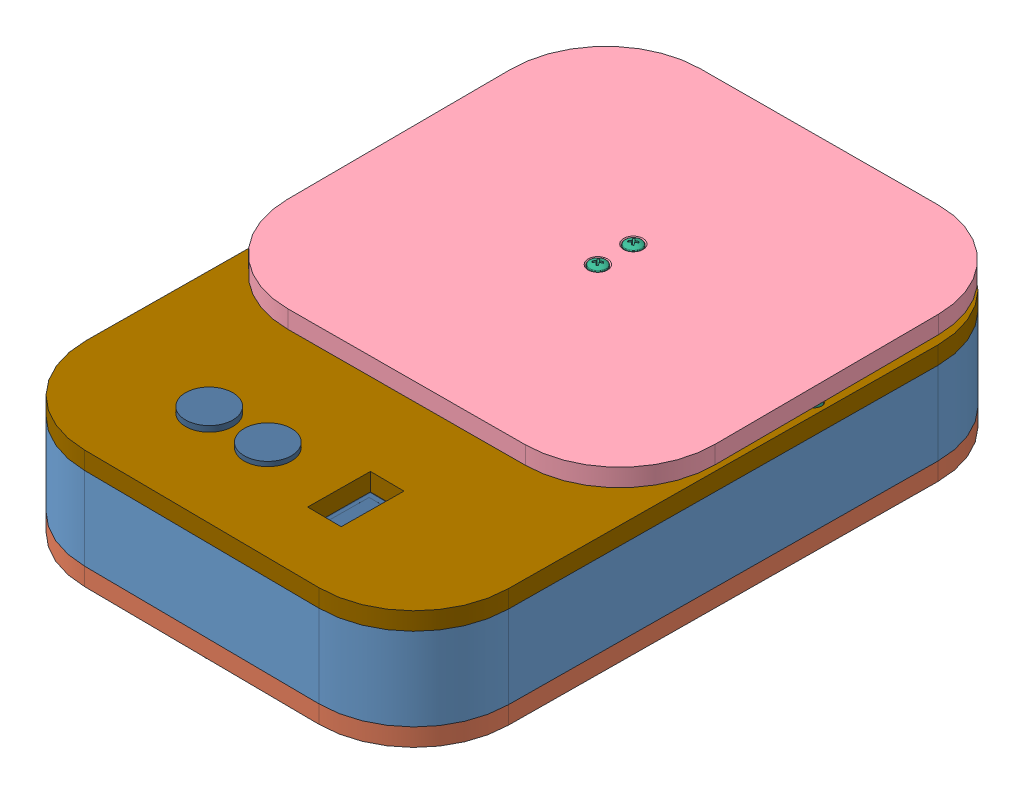
SolidWorks assembly Mainv2.0, configuration Default. Lengths in mm.
Overall size (189.49 80.65 261.56).
193 component instances, 46 part files, 22 mates.
Components (placement in the parent):
- Main-1: Main [Default] at (-331.7007 96.9527 454.1899) size (182.26 61.96 261.56)
  - mail wall-1: mail wall [Default] at (468.1099 74.0645 -181.95) x (-0.999962 0 -0.008727) z (0.008727 0 -0.999962) size (180 35 260)
  - bottom lid-2: bottom lid [Default] at (468.1099 31.5645 -181.95) x (0.999962 0 0.008727) z (-0.008727 0 0.999962) size (180 7.5 260)
  - Loadcell-1kg-No Name.step-1: Loadcell-1kg-No Name.step [Default] at (468.4825 94.8439 -197.5959) x (0 0 1) z (-1 0 0) size (91.8 14.23 13.91)
  - tray-1: tray [Default] at (468.6751 134.9439 -266.3463) x (0.999991 0 -0.00428) z (0.00428 0 0.999991) size (180 7.5 175)
  - Part5-1: Part5 [Default] at origin size (12.6 12.5 27.5)
  - pan cross head_am-1: pan cross head_am [B18.6.7M - M3.5 x 0.6 x 35 Type I Cross Recessed PHMS --35N] at (468.4825 128.4614 -232.8459) x (0 -1 0) z (-0.788636 0 0.61486) size (37.57 7 7)
  - pan cross head_am-3: pan cross head_am [B18.6.7M - M3.5 x 0.6 x 35 Type I Cross Recessed PHMS --35N] at (468.4825 128.5554 -217.8459) x (0 -1 0) z (0.792721 0 -0.609585) size (37.57 7 7)
  - Part1-1: Part1 [Default] at origin size (50 22.7 32.99)
  - hex bolt_am-1: hex bolt_am [B18.2.3.5M - Hex bolt M5 x 0.8 x 35 --16N] at (468.8184 72.2139 -162.6607) x (0 1 0) z (0 0 1) size (38.58 9.24 8)
  - hex bolt_am-2: hex bolt_am [B18.2.3.5M - Hex bolt M5 x 0.8 x 35 --16N] at (468.8184 72.2139 -177.7301) x (0 1 0) z (0 0 1) size (38.58 9.24 8)
  - Top lid with second pcb-2: Top lid with second pcb [Default] at (567.0429 -14.7467 22.0801) x (-0.999962 0 -0.008727) z (0.008727 0 -0.999962) size (180 18.64 260)
    - top lid-1: top lid [Default] at (100.7096 131.3112 203.159) size (180 7.5 260)
    - second_pcb.step-1: second_pcb.step [Default] at (17.5816 118.1729 -168.5329) x (0 0 -1) z (0 1 0) size (33.15 95 11)
    - Part64-1: Part64 [Default] at origin size (95.93 5.6 34.46)
    - pan cross head_am-2: pan cross head_am [B18.6.7M - M4 x 0.7 x 10 Type I Cross Recessed PHMS --10C] at (61.2696 114.6615 128.1391) x (0 1 0) z (0.253418 0 0.967357) size (13.07 8 8)
    - pan cross head_am-3: pan cross head_am [B18.6.7M - M4 x 0.7 x 10 Type I Cross Recessed PHMS --10C] at (152.2016 114.6615 127.7581) x (0 1 0) z (-0.971066 0 -0.238809) size (13.07 8 8)
    - pan cross head_am-4: pan cross head_am [B18.6.7M - M4 x 0.7 x 10 Type I Cross Recessed PHMS --10C] at (152.2016 114.6615 98.6751) x (0 1 0) z (-0.342128 0 -0.939653) size (13.07 8 8)
    - pan cross head_am-5: pan cross head_am [B18.6.7M - M4 x 0.7 x 10 Type I Cross Recessed PHMS --10C] at (61.2696 114.6615 98.6751) x (0 1 0) z (-0.923859 0 -0.382733) size (13.07 8 8)
- pcb_with_screws-1: pcb_with_screws [Default] at (347.1614 488.5879 -158.0964) x (0.371474 0 -0.928443) z (-0.928443 0 -0.371474) size (78.01 61.67 95.13)
  - pcb.step-1: pcb.step [Default] at (-541.6964 307.1593 96.7738) x (-0.93165 0 -0.363358) z (0 -1 0) size (48.01 79.98 16.61)
    - Board.step-1: Board.step [Default] at origin size (48.01 78.74 0.41)
      - Open CASCADE STEP translator 7.5 2.1.1.step-1: Open CASCADE STEP translator 7.5 2.1.1.step [Default] at (0 0 -0.4115) size (48.01 78.74 0.41)
    - HX711 out.step-1: HX711 out.step [Default] at origin size (10.16 2.54 10.59)
      - Header_4.step-1: Header_4.step [Default] at (27.685 46.598 -0.0051) x (0 -1 0) z (-1 0 0) size (2.54 10.59 10.16)
        - header.step-1: header.step [Default] at origin size (2.54 10.59 2.54)
          - header-0.step-1: header-0.step [Default] at origin size (2.54 8.5 2.54)
          - pin.step-1: pin.step [Default] at (-1.4 0 0) size (0.4 10 1.99)
        - header.step-2: header.step [Default] at (0 0 -2.54) size (2.54 10.59 2.54)
          - header-0.step-1: header-0.step [Default] at origin size (2.54 8.5 2.54)
          - pin.step-1: pin.step [Default] at (-1.4 0 0) size (0.4 10 1.99)
        - header.step-3: header.step [Default] at (0 0 -5.08) size (2.54 10.59 2.54)
          - header-0.step-1: header-0.step [Default] at origin size (2.54 8.5 2.54)
          - pin.step-1: pin.step [Default] at (-1.4 0 0) size (0.4 10 1.99)
        - header.step-4: header.step [Default] at (0 0 -7.62) size (2.54 10.59 2.54)
          - header-0.step-1: header-0.step [Default] at origin size (2.54 8.5 2.54)
          - pin.step-1: pin.step [Default] at (-1.4 0 0) size (0.4 10 1.99)
    - HX711_lc.step-1: HX711_lc.step [Default] at origin size (10.16 2.54 10.59)
      - Header_4.step-1: Header_4.step [Default] at (30.23 66.915 -0.0051) x (0 -1 0) z (-1 0 0) size (2.54 10.59 10.16)
        - header.step-1: header.step [Default] at origin size (2.54 10.59 2.54)
          - header-0.step-1: header-0.step [Default] at origin size (2.54 8.5 2.54)
          - pin.step-1: pin.step [Default] at (-1.4 0 0) size (0.4 10 1.99)
        - header.step-2: header.step [Default] at (0 0 -2.54) size (2.54 10.59 2.54)
          - header-0.step-1: header-0.step [Default] at origin size (2.54 8.5 2.54)
          - pin.step-1: pin.step [Default] at (-1.4 0 0) size (0.4 10 1.99)
        - header.step-3: header.step [Default] at (0 0 -5.08) size (2.54 10.59 2.54)
          - header-0.step-1: header-0.step [Default] at origin size (2.54 8.5 2.54)
          - pin.step-1: pin.step [Default] at (-1.4 0 0) size (0.4 10 1.99)
        - header.step-4: header.step [Default] at (0 0 -7.62) size (2.54 10.59 2.54)
          - header-0.step-1: header-0.step [Default] at origin size (2.54 8.5 2.54)
          - pin.step-1: pin.step [Default] at (-1.4 0 0) size (0.4 10 1.99)
    - usb 2.0.step-1: usb 2.0.step [Default] at origin size (7.8 5.5 3.71)
      - USB3090-30-A--3DModel-STEP-56544.step-1: USB3090-30-A--3DModel-STEP-56544.step [Default] at (7.762 1.514 0) x (1 0 0) z (0 -1 0) size (7.8 3.71 5.5)
    - R 470.step-1: R 470.step [Default] at origin size (2 1.25 0.6)
      - 6201218720.step-1: 6201218720.step [Default] at (15.687 7.62 0) x (1 0 0) z (0 0 1) size (2 1.25 0.6)
        - term1.step-1: term1.step [Default] at (-1 -0.625 0) size (0.35 1.25 0.6)
        - term2.step-1: term2.step [Default] at (0.65 -0.625 0) size (0.35 1.25 0.6)
        - body.step-1: body.step [Default] at (-0.65 -0.6125 0.006) size (1.3 1.22 0.59)
    - R 47k.step-1: R 47k.step [Default] at origin size (2 1.25 0.6)
      - 6062674512.step-1: 6062674512.step [Default] at (18.862 49.53 0) x (-1 0 0) z (0 0 1) size (2 1.25 0.6)
        - term1-1.step-1: term1-1.step [Default] at (-1 -0.625 0) size (0.35 1.25 0.6)
        - term2-2.step-1: term2-2.step [Default] at (0.65 -0.625 0) size (0.35 1.25 0.6)
        - body-3.step-1: body-3.step [Default] at (-0.65 -0.6125 0.006) size (1.3 1.22 0.59)
    - R 15k.step-1: R 15k.step [Default] at origin size (2 1.25 0.6)
      - 7267289360.step-1: 7267289360.step [Default] at (18.937 59.563 0) x (-1 0 0) z (0 0 1) size (2 1.25 0.6)
        - solidBody.step-1: solidBody.step [Default] at origin size (1.95 1.25 0.55)
        - Terminal.step-1: Terminal.step [Default] at origin size (2 1.25 0.6)
        - solidTop.step-1: solidTop.step [Default] at origin size (1.2 1.25 0.02)
    - R5-10K.step-1: R5-10K.step [Default] at origin size (1.6 0.8 0.55)
      - CRG0603F10K_10.step-1: CRG0603F10K_10.step [Default] at (45.212 17.526 0) x (1 0 0) z (0 -1 0) size (1.6 0.55 0.8)
    - R4-10K.step-1: R4-10K.step [Default] at origin size (1.6 0.8 0.55)
      - CRG0603F10K_10.step-1: CRG0603F10K_10.step [Default] at (45.212 22.7965 0) x (-1 0 0) z (0 1 0) size (1.6 0.55 0.8)
    - R3-10K.step-1: R3-10K.step [Default] at origin size (1.6 0.8 0.55)
      - CRG0603F10K_10.step-1: CRG0603F10K_10.step [Default] at (45.212 28.067 0) x (1 0 0) z (0 -1 0) size (1.6 0.55 0.8)
    - R 2k.step-1: R 2k.step [Default] at origin size (2 1.25 0.6)
      - 6062674512.step-1: 6062674512.step [Default] at (15.814 12.319 0) x (-1 0 0) z (0 0 1) size (2 1.25 0.6)
        - term1-1.step-1: term1-1.step [Default] at (-1 -0.625 0) size (0.35 1.25 0.6)
        - term2-2.step-1: term2-2.step [Default] at (0.65 -0.625 0) size (0.35 1.25 0.6)
        - body-3.step-1: body-3.step [Default] at (-0.65 -0.6125 0.006) size (1.3 1.22 0.59)
    - R2-10K.step-1: R2-10K.step [Default] at origin size (1.6 0.8 0.55)
      - CRG0603F10K_10.step-1: CRG0603F10K_10.step [Default] at (22.733 36.195 0) x (-1 0 0) z (0 1 0) size (1.6 0.55 0.8)
    - R1-10K.step-1: R1-10K.step [Default] at origin size (1.6 0.8 0.55)
      - CRG0603F10K_10.step-1: CRG0603F10K_10.step [Default] at (22.733 42.545 0) x (-1 0 0) z (0 1 0) size (1.6 0.55 0.8)
    - MCP73831.step-1: MCP73831.step [Default] at origin size (2.7 2.9 1.45)
      - MCP73831T-5ACI_OT.step-1: MCP73831T-5ACI_OT.step [Default] at (8.255 12.012 0) x (0 -1 0) z (-1 0 0) size (2.9 1.45 2.7)
    - LED.step-1: LED.step [Default] at origin size (3 1 2)
      - KPA-3010CGCK-Base.step-1: KPA-3010CGCK-Base.step [Default] at (16.51 1.651 0.508) x (-1 0 0) z (0 0 -1) size (2.16 1 1.02)
      - KPA-3010CGCK-Base-4.step-1: KPA-3010CGCK-Base-4.step [Default] at (16.51 1.651 0.508) x (-1 0 0) z (0 0 -1) size (3 1 1.22)
      - KPA-3010CGCK-Base-5.step-1: KPA-3010CGCK-Base-5.step [Default] at (16.51 1.651 0.508) x (-1 0 0) z (0 0 -1) size (0.9 1 0)
      - KPA-3010CGCK-Base-6.step-1: KPA-3010CGCK-Base-6.step [Default] at (16.51 1.651 0.508) x (-1 0 0) z (0 0 -1) size (0.8 1 0.02)
      - KPA-3010CGCK-Base-7.step-1: KPA-3010CGCK-Base-7.step [Default] at (16.51 1.651 0.508) x (-1 0 0) z (0 0 -1) size (2.96 1 0.96)
    - battery.step-1: battery.step [Default] at origin size (7.4 5.75 10.4)
      - 6062675712.step-1: 6062675712.step [Default] at (9.274 74.295 0) x (1 0 0) z (0 -1 0) size (7.4 10.4 5.75)
    - load cell.step-1: load cell.step [Default] at origin size (10.16 2.54 10.59)
      - Header_4.step-1: Header_4.step [Default] at (30.099 71.755 -0.0051) x (0 -1 0) z (-1 0 0) size (2.54 10.59 10.16)
        - header.step-1: header.step [Default] at origin size (2.54 10.59 2.54)
          - header-0.step-1: header-0.step [Default] at origin size (2.54 8.5 2.54)
          - pin.step-1: pin.step [Default] at (-1.4 0 0) size (0.4 10 1.99)
        - header.step-2: header.step [Default] at (0 0 -2.54) size (2.54 10.59 2.54)
          - header-0.step-1: header-0.step [Default] at origin size (2.54 8.5 2.54)
          - pin.step-1: pin.step [Default] at (-1.4 0 0) size (0.4 10 1.99)
        - header.step-3: header.step [Default] at (0 0 -5.08) size (2.54 10.59 2.54)
          - header-0.step-1: header-0.step [Default] at origin size (2.54 8.5 2.54)
          - pin.step-1: pin.step [Default] at (-1.4 0 0) size (0.4 10 1.99)
        - header.step-4: header.step [Default] at (0 0 -7.62) size (2.54 10.59 2.54)
          - header-0.step-1: header-0.step [Default] at origin size (2.54 8.5 2.54)
          - pin.step-1: pin.step [Default] at (-1.4 0 0) size (0.4 10 1.99)
    - buttons.step-1: buttons.step [Default] at origin size (2.54 10.16 10.59)
      - Header_4.step-1: Header_4.step [Default] at (39.497 59.817 -0.0051) x (-1 0 0) z (0 1 0) size (2.54 10.59 10.16)
        - header.step-1: header.step [Default] at origin size (2.54 10.59 2.54)
          - header-0.step-1: header-0.step [Default] at origin size (2.54 8.5 2.54)
          - pin.step-1: pin.step [Default] at (-1.4 0 0) size (0.4 10 1.99)
        - header.step-2: header.step [Default] at (0 0 -2.54) size (2.54 10.59 2.54)
          - header-0.step-1: header-0.step [Default] at origin size (2.54 8.5 2.54)
          - pin.step-1: pin.step [Default] at (-1.4 0 0) size (0.4 10 1.99)
        - header.step-3: header.step [Default] at (0 0 -5.08) size (2.54 10.59 2.54)
          - header-0.step-1: header-0.step [Default] at origin size (2.54 8.5 2.54)
          - pin.step-1: pin.step [Default] at (-1.4 0 0) size (0.4 10 1.99)
        - header.step-4: header.step [Default] at (0 0 -7.62) size (2.54 10.59 2.54)
          - header-0.step-1: header-0.step [Default] at origin size (2.54 8.5 2.54)
          - pin.step-1: pin.step [Default] at (-1.4 0 0) size (0.4 10 1.99)
    - OLED.step-1: OLED.step [Default] at origin size (2.54 10.16 16)
      - MTSW-104-22-S-S-420.step-1: MTSW-104-22-S-S-420.step [Default] at (44.831 57.277 0) x (0 -1 0) z (-1 0 0) size (10.16 16 2.54)
        - MTSW-104-22-S-420.step-1: MTSW-104-22-S-420.step [Default] at (0 -2.794 0) size (8.51 16 0.89)
        - MTSW-104-22-S-S-420_body.step-1: MTSW-104-22-S-S-420_body.step [Default] at origin size (10.16 2.54 2.54)
    - ESP-12F.step-1: ESP-12F.step [Default] at origin size (17.7 24.9 3.1)
      - ESP-12F-8.step-1: ESP-12F-8.step [Default] at (33.909 28.956 0) x (1 0 0) z (0 -1 0) size (17.7 3.1 24.9)
    - C5-4.7uF.step-1: C5-4.7uF.step [Default] at origin size (2 1.25 1.45)
      - 885012107013.step-1: 885012107013.step [Default] at (10.345 18.923 0) x (-1 0 0) z (0 0 1) size (2 1.25 1.45)
        - Fillet1.step-1: Fillet1.step [Default] at origin size (0.5 1.25 1.45)
        - Fillet2.step-1: Fillet2.step [Default] at origin size (0.5 1.25 1.45)
        - body2.step-1: body2.step [Default] at origin size (1 1.22 1.42)
    - C4-4.7uF.step-1: C4-4.7uF.step [Default] at origin size (2 1.25 1.45)
      - 885012107013.step-1: 885012107013.step [Default] at (11.245 26.543 0) x (1 0 0) z (0 0 1) size (2 1.25 1.45)
        - Fillet1.step-1: Fillet1.step [Default] at origin size (0.5 1.25 1.45)
        - Fillet2.step-1: Fillet2.step [Default] at origin size (0.5 1.25 1.45)
        - body2.step-1: body2.step [Default] at origin size (1 1.22 1.42)
    - C3-10uF.step-1: C3-10uF.step [Default] at origin size (5.3 4.5 5.5)
      - 865080340001.step-1: 865080340001.step [Default] at (10.737 64.643 0) x (-1 0 0) z (0 0 1) size (5.3 4.5 5.5)
        - Base.step-1: Base.step [Default] at origin size (4.5 4.5 1.6)
        - Pin1Fillet.step-1: Pin1Fillet.step [Default] at origin size (2.25 0.75 0.3)
        - Pin2Fillet.step-1: Pin2Fillet.step [Default] at origin size (2.25 0.75 0.3)
        - Fillet.step-1: Fillet.step [Default] at origin size (4.2 4.2 4.4)
      - 865080340001.step-2: 865080340001.step [Default] at (10.737 64.643 0) x (-1 0 0) z (0 0 1) size (5.3 4.5 5.5)
        - Base.step-1: Base.step [Default] at origin size (4.5 4.5 1.6)
        - Pin1Fillet.step-1: Pin1Fillet.step [Default] at origin size (2.25 0.75 0.3)
        - Pin2Fillet.step-1: Pin2Fillet.step [Default] at origin size (2.25 0.75 0.3)
        - Fillet.step-1: Fillet.step [Default] at origin size (4.2 4.2 4.4)
    - C2-10uF.step-1: C2-10uF.step [Default] at origin size (5.3 4.5 5.5)
      - 865080340001.step-1: 865080340001.step [Default] at (10.737 44.069 0) x (-1 0 0) z (0 0 1) size (5.3 4.5 5.5)
        - Base.step-1: Base.step [Default] at origin size (4.5 4.5 1.6)
        - Pin1Fillet.step-1: Pin1Fillet.step [Default] at origin size (2.25 0.75 0.3)
        - Pin2Fillet.step-1: Pin2Fillet.step [Default] at origin size (2.25 0.75 0.3)
        - Fillet.step-1: Fillet.step [Default] at origin size (4.2 4.2 4.4)
      - 865080340001.step-2: 865080340001.step [Default] at (10.737 44.069 0) x (-1 0 0) z (0 0 1) size (5.3 4.5 5.5)
        - Base.step-1: Base.step [Default] at origin size (4.5 4.5 1.6)
        - Pin1Fillet.step-1: Pin1Fillet.step [Default] at origin size (2.25 0.75 0.3)
        - Pin2Fillet.step-1: Pin2Fillet.step [Default] at origin size (2.25 0.75 0.3)
        - Fillet.step-1: Fillet.step [Default] at origin size (4.2 4.2 4.4)
    - C1-10uF.step-1: C1-10uF.step [Default] at origin size (5.3 4.5 5.5)
      - 865080340001.step-1: 865080340001.step [Default] at (33.583 11.303 0) x (-1 0 0) z (0 0 1) size (5.3 4.5 5.5)
        - Base.step-1: Base.step [Default] at origin size (4.5 4.5 1.6)
        - Pin1Fillet.step-1: Pin1Fillet.step [Default] at origin size (2.25 0.75 0.3)
        - Pin2Fillet.step-1: Pin2Fillet.step [Default] at origin size (2.25 0.75 0.3)
        - Fillet.step-1: Fillet.step [Default] at origin size (4.2 4.2 4.4)
      - 865080340001.step-2: 865080340001.step [Default] at (33.583 11.303 0) x (-1 0 0) z (0 0 1) size (5.3 4.5 5.5)
        - Base.step-1: Base.step [Default] at origin size (4.5 4.5 1.6)
        - Pin1Fillet.step-1: Pin1Fillet.step [Default] at origin size (2.25 0.75 0.3)
        - Pin2Fillet.step-1: Pin2Fillet.step [Default] at origin size (2.25 0.75 0.3)
        - Fillet.step-1: Fillet.step [Default] at origin size (4.2 4.2 4.4)
    - TC2117.step-1: TC2117.step [Default] at origin size (7.13 5.32 1.17)
      - TC2117-3.3VDBTR.step-1: TC2117-3.3VDBTR.step [Default] at (10.864 54.356 0) x (-1 0 0) z (0 0 1) size (7 5.32 1.17)
        - body.step-1: body.step [Default] at origin size (1.3 1.22 0.59)
        - PinsArrayL.step-1: PinsArrayL.step [Default] at origin size (1.75 5.32 1.17)
        - FilletPinR.step-1: FilletPinR.step [Default] at origin size (1.75 3 1.17)
      - TC2117-3.3VDBTR.step-2: TC2117-3.3VDBTR.step [Default] at (10.737 54.356 0) x (-1 0 0) z (0 0 1) size (7 5.32 1.17)
        - body.step-1: body.step [Default] at origin size (1.3 1.22 0.59)
        - PinsArrayL.step-1: PinsArrayL.step [Default] at origin size (1.75 5.32 1.17)
        - FilletPinR.step-1: FilletPinR.step [Default] at origin size (1.75 3 1.17)
  - Part36-1: Part36 [Default] at (-868.0076 716.489 235.6311) x (0.932186 0.214397 0.291656) z (-0.265595 0.952553 0.148668) size (53.08 79 35.65)
  - pan cross head_am-4: pan cross head_am [B18.6.7M - M2.5 x 0.45 x 5 Type I Cross Recessed PHMS --5N] at (-581.9119 305.0593 74.4096) x (0 1 0) z (-0.92188 0 0.387475) size (7.07 5 5)
  - pan cross head_am-5: pan cross head_am [B18.6.7M - M2.5 x 0.45 x 5 Type I Cross Recessed PHMS --5N] at (-556.4391 305.0593 9.0972) x (0 1 0) z (-0.72878 0 -0.684748) size (7.07 5 5)
  - pan cross head_am-6: pan cross head_am [B18.6.7M - M2.5 x 0.45 x 5 Type I Cross Recessed PHMS --5N] at (-515.9277 305.0593 24.761) x (0 1 0) z (0.615507 0 -0.788131) size (7.07 5 5)
  - pan cross head_am-7: pan cross head_am [B18.6.7M - M2.5 x 0.45 x 5 Type I Cross Recessed PHMS --5N] at (-541.4467 305.0593 90.1917) x (0 1 0) z (-0.986634 0 -0.162951) size (7.07 5 5)
- Part37^Mainv2.0-1: Part37^Mainv2.0 [Default] at (232.9335 200.1845 720.6732) x (-0.999475 0 0.032385) z (0 1 0) size (19.97 19.97 10) (virtual)
- Part37^Mainv2.0-2: Part37^Mainv2.0 [Default] at (177.4351 200.668 728.4104) x (-0.998664 0 -0.051668) z (0 1 0) size (19.97 19.97 10) (virtual)
- pan cross head_am-3: pan cross head_am [B18.6.7M - M3 x 0.5 x 16 Type I Cross Recessed PHMS --16C] at (137.5058 161.1172 146.5823) x (0 1 0) z (0 0 1) size (18.37 5.6 5.6)
- pan cross head_am-4: pan cross head_am [B18.6.7M - M3 x 0.5 x 16 Type I Cross Recessed PHMS --16C] at (50.1199 161.1172 271.4869) x (0 1 0) z (0 0 1) size (18.37 5.6 5.6)
- pan cross head_am-7: pan cross head_am [B18.6.7M - M3 x 0.5 x 16 Type I Cross Recessed PHMS --16C] at (222.0917 161.1172 272.9876) x (0 1 0) z (0 0 1) size (18.37 5.6 5.6)
- pan cross head_am-9: pan cross head_am [B18.6.7M - M3 x 0.5 x 16 Type I Cross Recessed PHMS --16C] at (135.3113 161.1172 398.0567) x (0 1 0) z (0 0 1) size (18.37 5.6 5.6)
- pan cross head_am-11: pan cross head_am [B18.6.7M - M3 x 0.5 x 16 Type I Cross Recessed PHMS --16C] at (52.0363 215.7083 230.7075) x (0 -1 0) z (0.190223 0 -0.981741) size (18.37 5.6 5.6)
- pan cross head_am-13: pan cross head_am [B18.6.7M - M3 x 0.5 x 16 Type I Cross Recessed PHMS --16C] at (221.8864 215.4097 229.9805) x (0 -1 0) z (-0.613644 0 -0.789583) size (18.37 5.6 5.6)
- pan cross head_am-14: pan cross head_am [B18.6.7M - M3 x 0.5 x 16 Type I Cross Recessed PHMS --16C] at (137.5433 215.6271 147.9494) x (0 -1 0) z (0.848821 0 -0.52868) size (18.37 5.6 5.6)
Mates (geometry in assembly coordinates):
- Coincident1: coincident anti-aligned: plane of Main-1/bottom lid-2 through (85.6258 171.0172 361.8002) normal (0 1 0); circle of pcb_with_screws-1/Part36-1
- Coincident2: coincident anti-aligned: plane of Main-1/mail wall-1 through (55.3651 206.0172 391.5372) normal (0.999962 0 0.008727); plane of pcb_with_screws-1/pcb.step-1/Board.step-1/Open CASCADE STEP translator 7.5 2.1.1.step-1 through (56.0864 181.0172 308.8891) normal (-0.999962 0 -0.008727)
- Lock1: lock: unknown of Main-1/bottom lid-2; unknown of pcb_with_screws-1/Part36-1
- Concentric4: concentric anti-aligned: circle of Main-1/top lid-1; circle of Part37^Mainv1.1-2
- Concentric5: concentric anti-aligned: circle of Main-1/top lid-1; circle of Part37^Mainv1.1-1
- Concentric7: concentric aligned: cylinder of Main-1/bottom lid-2 through (222.0917 163.5172 272.9876) axis (0 -1 0) radius 1.7; cylinder of pan cross head_am-4 through (222.0917 109.9845 272.9876) axis (0 -1 0) radius 1.5
- Concentric8: concentric anti-aligned: circle of Main-1/Top lid with second pcb-2/top lid-1; circle of Part37^Mainv2.0-1
- Concentric9: concentric anti-aligned: circle of Main-1/Top lid with second pcb-2/top lid-1; circle of Part37^Mainv2.0-2
- Concentric10: concentric anti-aligned: cone of Main-1/bottom lid-2 through (137.5058 163.5172 146.5823) axis (0 1 0); cylinder of pan cross head_am-3 through (137.5058 135.7172 146.5823) axis (0 -1 0) radius 2.8
- Coincident4: coincident anti-aligned: plane of Main-1/bottom lid-2 through (85.6258 163.5172 361.8002) normal (0 -1 0); plane of pan cross head_am-3 through (136.0058 163.5172 146.5823) normal (0 1 0)
- Concentric11: concentric anti-aligned: cone of Main-1/bottom lid-2 through (50.1199 163.5172 271.4869) axis (0 1 0); cylinder of pan cross head_am-4 through (50.1199 135.7172 271.4869) axis (0 -1 0) radius 2.8
- Coincident5: coincident anti-aligned: plane of Main-1/bottom lid-2 through (85.6258 163.5172 361.8002) normal (0 -1 0); plane of pan cross head_am-4 through (48.6199 163.5172 271.4869) normal (0 1 0)
- Concentric12: concentric anti-aligned: cone of Main-1/bottom lid-2 through (222.0917 163.5172 272.9876) axis (0 1 0); cylinder of pan cross head_am-7 through (222.0917 135.7172 272.9876) axis (0 -1 0) radius 2.8
- Coincident6: coincident anti-aligned: plane of Main-1/bottom lid-2 through (85.6258 163.5172 361.8002) normal (0 -1 0); plane of pan cross head_am-7 through (220.5917 163.5172 272.9876) normal (0 1 0)
- Concentric13: concentric anti-aligned: cone of Main-1/bottom lid-2 through (135.3113 163.5172 398.0567) axis (0 1 0); cylinder of pan cross head_am-9 through (135.3113 135.7172 398.0567) axis (0 -1 0) radius 2.8
- Coincident7: coincident anti-aligned: plane of Main-1/bottom lid-2 through (85.6258 163.5172 361.8002) normal (0 -1 0); plane of pan cross head_am-9 through (133.8113 163.5172 398.0567) normal (0 1 0)
- Concentric16: concentric aligned: cylinder of Main-1/mail wall-1 through (52.0363 213.5172 230.7075) axis (0 1 0) radius 1.7; cylinder of pan cross head_am-11 through (52.0363 241.1083 230.7075) axis (0 1 0) radius 1.5
- Concentric18: concentric anti-aligned: cone of Main-1/Top lid with second pcb-2/top lid-1 through (137.5433 213.5172 147.9494) axis (0 -1 0); cylinder of pan cross head_am-14 through (137.5433 241.0271 147.9494) axis (0 1 0) radius 2.8
- Concentric19: concentric aligned: circle of Main-1/Top lid with second pcb-2/top lid-1; cylinder of pan cross head_am-13 through (221.8864 240.8097 229.9805) axis (0 1 0) radius 2.8
- Screw1: screw = 5 aligned: cylinder of Main-1/Top lid with second pcb-2/top lid-1 through (52.0363 213.5172 230.7075) axis (0 1 0) radius 1.7; cylinder of pan cross head_am-11 through (52.0363 241.1083 230.7075) axis (0 1 0) radius 1.5
- Screw2: screw = 5 aligned: cylinder of Main-1/Top lid with second pcb-2/top lid-1 through (137.5433 213.5172 147.9494) axis (0 1 0) radius 1.7; cylinder of pan cross head_am-14 through (137.5433 241.0271 147.9494) axis (0 1 0) radius 1.5
- Screw3: screw = 5 aligned: cylinder of Main-1/Top lid with second pcb-2/top lid-1 through (221.8864 213.5172 229.9805) axis (0 1 0) radius 1.7; cylinder of pan cross head_am-13 through (221.8864 240.8097 229.9805) axis (0 1 0) radius 1.5
